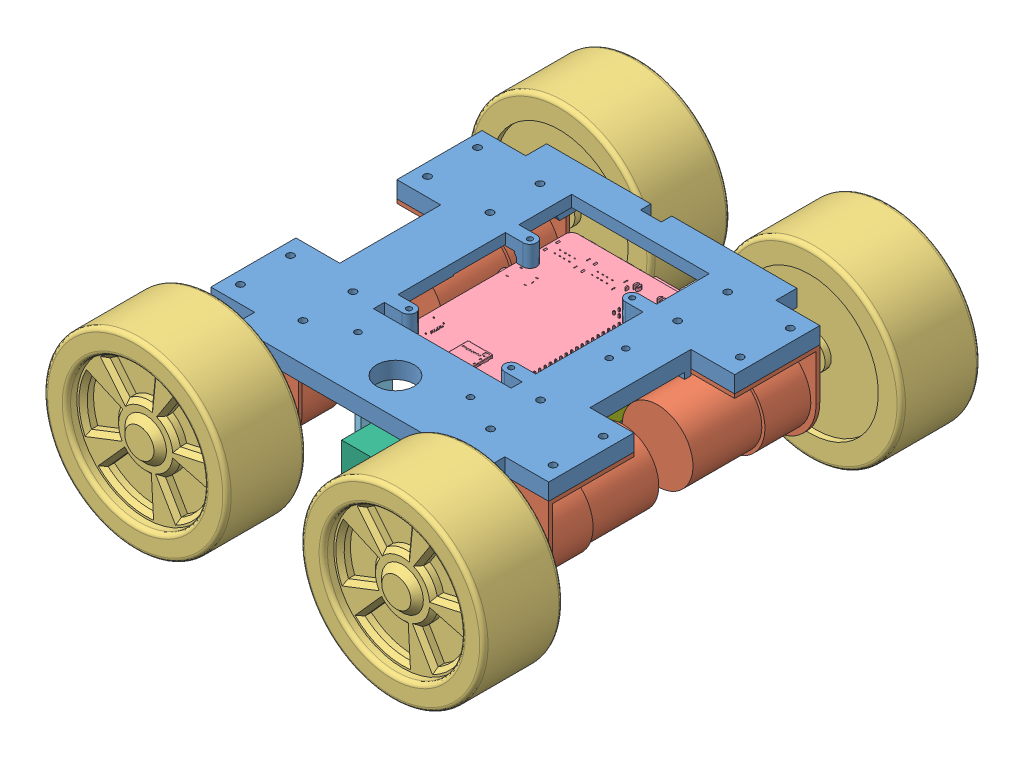
SolidWorks assembly 装配体, configuration Default. Lengths in mm.
Overall size (211.48 94.96 238.16).
13 component instances, 7 part files, 31 mates.
Components (placement in the parent):
- 底盘-1: 底盘 [默认] at origin size (162 11 150)
- 电机-1: 电机 [默认] at (-60 -24 -41.2) x (1 0 0) z (0 -1 0) size (42 75.8 45)
- 车轮-1: 车轮 [默认] at (-60 -22.2 -81.08) x (0.996587 0.082554 0) z (-0.082554 0.996587 0) size (88 38 88)
- 电机-2: 电机 [默认] at (-60 -24 41.2) x (-1 0 0) z (0 -1 0) size (42 75.8 45)
- raspberry 4b-1: raspberry 4b [Standard] at (-16.7793 22.0544 -80.9668) x (0 0 -1) z (0 -1 0) size (90.11 58.5 18.59)
- 电池架-1: 电池架 [默认] at (0 -50 56) x (0 0 -1) z (1 0 0) size (15 53 66)
- 电池-1: 电池 [默认] at (-0.0878 -50 11.2055) x (0 0 -1) z (1 0 0) size (110 27 34)
- 电池托架-1: 电池托架 [默认] at (44 -3 -4.984) x (0 0 -1) z (1 0 0) size (57.98 53 57)
- 车轮-2: 车轮 [默认] at (-63.188 -21.7285 81.08) x (1 0 0) z (0 -1 0) size (88 38 88)
- 电机-3: 电机 [默认] at (60 -24 -41.2) x (1 0 0) z (0 -1 0) size (42 75.8 45)
- 电机-4: 电机 [默认] at (60 -24 41.2) x (-1 0 0) z (0 -1 0) size (42 75.8 45)
- 车轮-3: 车轮 [默认] at (60 -22.2 81.08) x (1 0 0) z (0 -1 0) size (88 38 88)
- 车轮-4: 车轮 [默认] at (60 -22.2 -81.08) x (1 0 0) z (0 1 0) size (88 38 88)
Mates (geometry in assembly coordinates):
- 同心1: concentric anti-aligned: circle of 底盘-1; circle of 电机-1
- 同心2: concentric anti-aligned: circle of 底盘-1; circle of 电机-1
- 重合3: coincident anti-aligned: plane of 底盘-1 through (0 0 0) normal (0 -1 0); plane of 电机-1 through (-39 0 -65) normal (0 1 0)
- 平行1: parallel aligned: plane of 电机-1 through (-60 -22.2 -84) normal (0 0 -1); plane of 车轮-1 through (-60 -22.2 -117.08) normal (0 0 -1)
- 同心3: concentric aligned: circle of 电机-1; circle of 车轮-1
- 重合5: coincident anti-aligned: plane of 电机-1 through (-60 -22.2 -84) normal (0 0 -1); plane of 车轮-1 through (-60 -22.2 -84) normal (0 0 1)
- 同心4: concentric anti-aligned: circle of 底盘-1; circle of 电机-2
- 同心5: concentric anti-aligned: circle of 底盘-1; circle of 电机-2
- 重合8: coincident anti-aligned: plane of 底盘-1 through (0 0 0) normal (0 -1 0); plane of 电机-2 through (-81 0 65) normal (0 1 0)
- 同心6: concentric aligned: circle of 底盘-1; circle of raspberry 4b-1
- 同心7: concentric aligned: circle of 底盘-1; circle of raspberry 4b-1
- 重合9: coincident anti-aligned: plane of 底盘-1 through (24.5 -2 -31.5) normal (0 -1 0); plane of raspberry 4b-1 through (-25 -2 -52) normal (0 1 0)
- 重合10: coincident anti-aligned: plane of 底盘-1 through (0 0 0) normal (0 -1 0); plane of 电池架-1 through (-18 0 41) normal (0 1 0)
- 平行2: parallel aligned: plane of 底盘-1 through (-60 8 75) normal (0 0 1); plane of 电池架-1 through (0 -50 56) normal (0 0 1)
- 平行3: parallel aligned: plane of 电池架-1 through (21 -53 41) normal (1 0 0); plane of 电池-1 through (16.9122 -23 66.2055) normal (1 0 0)
- 平行4: parallel aligned: plane of 电池架-1 through (0 -53 41) normal (0 -1 0); plane of 电池-1 through (-0.0878 -50 11.2055) normal (0 -1 0)
- 重合14: coincident anti-aligned: plane of 电池架-1 through (0 -50 41) normal (0 1 0); plane of 电池-1 through (-0.0878 -50 11.2055) normal (0 -1 0)
- 同心8: concentric anti-aligned: circle of 底盘-1; circle of 电池架-1
- 重合15: coincident anti-aligned: plane of 底盘-1 through (0 0 0) normal (0 -1 0); plane of 电池托架-1 through (44 0 -4.984) normal (0 1 0)
- 平行5: parallel aligned: plane of 底盘-1 through (60 8 -75) normal (1 0 0); plane of 电池托架-1 through (49 0 5.016) normal (1 0 0)
- 重合18: coincident aligned: plane of 底盘-1 through (36 -3 -65) normal (-1 0 0); plane of 电池托架-1 through (36 -23 -14.984) normal (-1 0 0)
- 同心12: concentric aligned: circle of 底盘-1; circle of 电池托架-1
- 重合19: coincident anti-aligned: plane of 电机-2 through (-60 -22.2 84) normal (0 0 1); plane of 车轮-2 through (-63.188 -21.7285 84) normal (0 0 -1)
- 重合20: coincident anti-aligned: circle of 底盘-1; circle of 电机-3
- 重合21: coincident anti-aligned: circle of 底盘-1; circle of 电机-3
- 重合22: coincident anti-aligned: circle of 底盘-1; circle of 电机-4
- 重合23: coincident anti-aligned: circle of 底盘-1; circle of 电机-4
- 重合25: coincident anti-aligned: circle of 电机-4; plane of 车轮-3 through (60 -22.2 84) normal (0 0 -1)
- 重合26: coincident anti-aligned: circle of 电机-3; circle of 车轮-4
- 重合27: coincident anti-aligned: plane of 电机-4 through (60 -22.2 84) normal (0 0 1); plane of 车轮-3 through (60 -22.2 84) normal (0 0 -1)
- 同心13: concentric anti-aligned: circle of 电机-4; circle of 车轮-3
